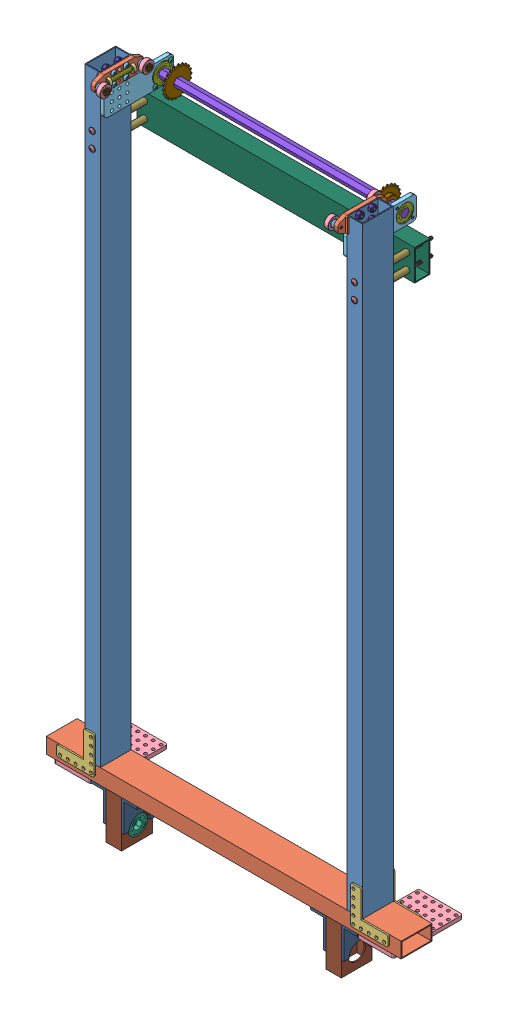
SolidWorks assembly Assem1^short elevator(1), configuration Default. Lengths in mm.
Overall size (584.2 1114.95 169.19).
89 component instances, 24 part files, 69 mates.
Components (placement in the parent):
- 2x1 extrude-1: 2x1 extrude [Default] at (149.0883 176.1618 1108.344) size (25.4 990.6 50.8)
- 2x1 extrude-2: 2x1 extrude [Default] at (580.8883 176.1618 1108.344) size (25.4 990.6 50.8)
- 2x1 23in extrude-1: 2x1 23in extrude [Default] at (669.7883 150.7618 1057.544) x (0 -1 0) z (-1 0 0) size (25.4 50.8 584.2)
- 90Degree L-1: 90Degree L [Default] at (147.322 -398.8739 726.1446) x (0 -1 0) z (-0.754511 0 0.656287) size (61.93 42.53 48.36)
- 90Degree L-2: 90Degree L [Default] at (147.322 -398.8739 779.4446) x (0 -1 0) z (-0.754511 0 0.656287) size (61.93 42.53 48.36)
- 90Degree L-3: 90Degree L [Default] at (31.2526 177.9281 726.1446) x (-1 0 0) z (0 0.754511 0.656287) size (61.93 42.53 48.36)
- 90Degree L-4: 90Degree L [Default] at (31.2526 177.9281 779.4446) x (-1 0 0) z (0 0.754511 0.656287) size (61.93 42.53 48.36)
- elevator motor mount-1: elevator motor mount [Default] at (724.1239 177.9281 1386.4435) x (1 0 0) z (0 0.754511 -0.656287) size (73.03 90.18 79.54)
- elevator motor mount-2: elevator motor mount [Default] at (31.2526 117.5955 1386.4435) x (-1 0 0) z (0 -0.754511 -0.656287) size (73.03 90.18 79.54)
- Copy of axle bracket^Assem1_short elevator(1)-2: Copy of axle bracket^Assem1_short elevator(1) [Default] at (-511.8423 2761.443 1667.3239) x (0.041389 -0.998995 -0.017175) z (0.999131 0.041466 -0.004112) size (40.43 115.12 11.68) (virtual)
  - Top Elevator Bearing Plate - ELEV-DRIVE-002.step-1: Top Elevator Bearing Plate - ELEV-DRIVE-002.step [Default] at (533.5722 545.5094 1067.8534) x (-0.017175 -0.999844 -0.004112) z (0.041389 -0.00482 0.999131) size (114.3 38.1 6.35)
  - 91255A191_Button Head Hex Drive Screw (1).step-1: 91255A191_Button Head Hex Drive Screw (1).step [Default] at (1706.7511 633.6223 1020.9438) x (-0.998995 0.01699 0.041466) z (-0.041389 0.00482 -0.999131) size (7.92 7.92 10.15)
  - 91255A191_Button Head Hex Drive Screw (1).step-2: 91255A191_Button Head Hex Drive Screw (1).step [Default] at (1680.7252 608.4497 1021.9005) x (-0.998995 0.01699 0.041466) z (-0.041389 0.00482 -0.999131) size (7.92 7.92 10.15)
  - TTB-0001_HalfInchHexBearing.step-1: TTB-0001_HalfInchHexBearing.step [Default] at (1693.9487 621.0115 1026.5041) x (-0.952853 -0.301042 0.03802) z (0.300597 -0.953599 -0.017053) size (31.12 7.94 31.12)
- Copy of Copy of Assem12^Assem1_short elevator(1)-2: Copy of Copy of Assem12^Assem1_short elevator(1) [Default] at (1267.2189 -516.8194 1667.3239) x (-0.041389 0.998995 -0.017175) z (-0.999131 -0.041466 -0.004112) size (40.43 115.12 11.68) (virtual)
  - Top Elevator Bearing Plate - ELEV-DRIVE-002.step-1: Top Elevator Bearing Plate - ELEV-DRIVE-002.step [Default] at (533.5722 545.5094 1067.8534) x (-0.017175 -0.999844 -0.004112) z (0.041389 -0.00482 0.999131) size (114.3 38.1 6.35)
  - 91255A191_Button Head Hex Drive Screw (1).step-1: 91255A191_Button Head Hex Drive Screw (1).step [Default] at (1706.7511 633.6223 1020.9438) x (-0.998995 0.01699 0.041466) z (-0.041389 0.00482 -0.999131) size (7.92 7.92 10.15)
  - 91255A191_Button Head Hex Drive Screw (1).step-2: 91255A191_Button Head Hex Drive Screw (1).step [Default] at (1680.7252 608.4497 1021.9005) x (-0.998995 0.01699 0.041466) z (-0.041389 0.00482 -0.999131) size (7.92 7.92 10.15)
  - TTB-0001_HalfInchHexBearing.step-1: TTB-0001_HalfInchHexBearing.step [Default] at (1693.9487 621.0115 1026.5041) x (-0.952853 -0.301042 0.03802) z (0.300597 -0.953599 -0.017053) size (31.12 7.94 31.12)
- 16in .5 hex axle-1: 16in .5 hex axle [Default] at (580.8883 1126.5392 1025.6307) x (0 0.397978 0.917395) z (-1 0 0) size (14.35 13.94 406.4)
- 22t 25chain gear-1: 22t 25chain gear [Default] at (698.6259 1091.6339 2219.5137) x (1 0 0) z (0 -0.367143 -0.930165) size (9.18 48.36 48.44)
- 22t 25chain gear-2: 22t 25chain gear [Default] at (56.7864 420.9907 1995.199) x (-1 0 0) z (0 0.852889 -0.522092) size (9.18 48.36 48.44)
- Copy of Copy (2) of Assem13^Assem1_short elevator(1)-2: Copy of Copy (2) of Assem13^Assem1_short elevator(1) [Default] at (-330.6974 177.9281 779.4446) x (-1 0 0) z (0 0.754511 0.656287) size (76.2 88.34 90.83) (virtual)
  - 1x2x2 L bracket-1: 1x2x2 L bracket [Default] at (-550.7787 227.658 162.0158) x (0 0.754511 0.656287) z (-1 0 0) size (50.8 50.8 25.4)
  - 1x2x3-1: 1x2x3 [Default] at (-514.7107 227.658 162.0158) x (-1 0 0) z (0 -0.754511 -0.656287) size (25.4 76.2 50.8)
  - 1x2x2 L bracket-2: 1x2x2 L bracket [Default] at (-504.0427 265.9872 195.3552) x (0 -0.754511 -0.656287) z (1 0 0) size (50.8 50.8 25.4)
- Copy of Copy of Assem13^Assem1_short elevator(1)-2: Copy of Copy of Assem13^Assem1_short elevator(1) [Default] at (31.2526 177.9281 779.4446) x (-1 0 0) z (0 0.754511 0.656287) size (76.2 88.34 90.83) (virtual)
  - 1x2x2 L bracket-1: 1x2x2 L bracket [Default] at (-550.7787 227.658 162.0158) x (0 0.754511 0.656287) z (-1 0 0) size (50.8 50.8 25.4)
  - 1x2x3-1: 1x2x3 [Default] at (-514.7107 227.658 162.0158) x (-1 0 0) z (0 -0.754511 -0.656287) size (25.4 76.2 50.8)
  - 1x2x2 L bracket-2: 1x2x2 L bracket [Default] at (-504.0427 265.9872 195.3552) x (0 -0.754511 -0.656287) z (1 0 0) size (50.8 50.8 25.4)
- Copy of Copy of Assem15^Assem1_short elevator(1)-2: Copy of Copy of Assem15^Assem1_short elevator(1) [Default] at (1830.9432 2239.2418 1667.3239) x (-0.916906 -0.398734 -0.017175) z (0.398855 -0.917005 -0.004112) size (13.77 134.77 13.77) (virtual)
  - 1.375in Long Aluminum Spacer for Crossbar ELEV-DRIVE-008.step-1: 1.375in Long Aluminum Spacer for Crossbar ELEV-DRIVE-008.step [Default] at (1618.2207 579.6208 597.2661) x (0.999819 -0.017141 -0.008284) z (0.008213 -0.004254 0.999957) size (9.53 34.92 9.53)
  - 5 Inch Long 10-32 Screw 287951.step-1: 5 Inch Long 10-32 Screw 287951.step [Default] at (1618.4098 590.63 597.3114) x (0.999851 -0.017183 0.001798) z (-0.017175 -0.999844 -0.004112) size (11.43 13.19 134.54)
  - 91831A411_18-8 Stainless Steel Nylon-Insert Locknut (2).step-1: 91831A411_18-8 Stainless Steel Nylon-Insert Locknut (2).step [Default] at (1619.2568 639.9364 597.5142) x (0.999849 -0.017186 0.002623) z (-0.002693 -0.004067 0.999988) size (9.53 5.96 11)
- Copy of Copy (2) of Assem15^Assem1_short elevator(1)-2: Copy of Copy (2) of Assem15^Assem1_short elevator(1) [Default] at (1830.9432 2264.6418 1667.3239) x (-0.916906 -0.398734 -0.017175) z (0.398855 -0.917005 -0.004112) size (13.77 134.77 13.77) (virtual)
  - 1.375in Long Aluminum Spacer for Crossbar ELEV-DRIVE-008.step-1: 1.375in Long Aluminum Spacer for Crossbar ELEV-DRIVE-008.step [Default] at (1618.2207 579.6208 597.2661) x (0.999819 -0.017141 -0.008284) z (0.008213 -0.004254 0.999957) size (9.53 34.92 9.53)
  - 5 Inch Long 10-32 Screw 287951.step-1: 5 Inch Long 10-32 Screw 287951.step [Default] at (1618.4098 590.63 597.3114) x (0.999851 -0.017183 0.001798) z (-0.017175 -0.999844 -0.004112) size (11.43 13.19 134.54)
  - 91831A411_18-8 Stainless Steel Nylon-Insert Locknut (2).step-1: 91831A411_18-8 Stainless Steel Nylon-Insert Locknut (2).step [Default] at (1619.2568 639.9364 597.5142) x (0.999849 -0.017186 0.002623) z (-0.002693 -0.004067 0.999988) size (9.53 5.96 11)
- Copy of Copy (3) of Assem15^Assem1_short elevator(1)-2: Copy of Copy (3) of Assem15^Assem1_short elevator(1) [Default] at (1399.1432 2239.2418 1667.3239) x (-0.916906 -0.398734 -0.017175) z (0.398855 -0.917005 -0.004112) size (13.77 134.77 13.77) (virtual)
  - 1.375in Long Aluminum Spacer for Crossbar ELEV-DRIVE-008.step-1: 1.375in Long Aluminum Spacer for Crossbar ELEV-DRIVE-008.step [Default] at (1618.2207 579.6208 597.2661) x (0.999819 -0.017141 -0.008284) z (0.008213 -0.004254 0.999957) size (9.53 34.92 9.53)
  - 5 Inch Long 10-32 Screw 287951.step-1: 5 Inch Long 10-32 Screw 287951.step [Default] at (1618.4098 590.63 597.3114) x (0.999851 -0.017183 0.001798) z (-0.017175 -0.999844 -0.004112) size (11.43 13.19 134.54)
  - 91831A411_18-8 Stainless Steel Nylon-Insert Locknut (2).step-1: 91831A411_18-8 Stainless Steel Nylon-Insert Locknut (2).step [Default] at (1619.2568 639.9364 597.5142) x (0.999849 -0.017186 0.002623) z (-0.002693 -0.004067 0.999988) size (9.53 5.96 11)
- Copy of Copy (4) of Assem15^Assem1_short elevator(1)-2: Copy of Copy (4) of Assem15^Assem1_short elevator(1) [Default] at (1399.1432 2264.6418 1667.3239) x (-0.916906 -0.398734 -0.017175) z (0.398855 -0.917005 -0.004112) size (13.77 134.77 13.77) (virtual)
  - 1.375in Long Aluminum Spacer for Crossbar ELEV-DRIVE-008.step-1: 1.375in Long Aluminum Spacer for Crossbar ELEV-DRIVE-008.step [Default] at (1618.2207 579.6208 597.2661) x (0.999819 -0.017141 -0.008284) z (0.008213 -0.004254 0.999957) size (9.53 34.92 9.53)
  - 5 Inch Long 10-32 Screw 287951.step-1: 5 Inch Long 10-32 Screw 287951.step [Default] at (1618.4098 590.63 597.3114) x (0.999851 -0.017183 0.001798) z (-0.017175 -0.999844 -0.004112) size (11.43 13.19 134.54)
  - 91831A411_18-8 Stainless Steel Nylon-Insert Locknut (2).step-1: 91831A411_18-8 Stainless Steel Nylon-Insert Locknut (2).step [Default] at (1619.2568 639.9364 597.5142) x (0.999849 -0.017186 0.002623) z (-0.002693 -0.004067 0.999988) size (9.53 5.96 11)
- 2x1 18in extrude-1: 2x1 18in extrude [Default] at (149.0883 1090.5618 997.219) x (1 0 0) z (0 -1 0) size (457.2 25.4 50.8)
- Copy of Copy of Assem10^Assem1_short elevator(1)-2: Copy of Copy of Assem10^Assem1_short elevator(1) [Default] at (-527.4189 487.9 -235.3019) x (-1 0 0) z (0 1 0) size (31.06 89.43 29.43) (virtual)
  - Sliding Elevator Bearing Block Kit.step-1: Sliding Elevator Bearing Block Kit.step [Default] at (-2.279 1755.626 148.4607) x (0 -0.999847 -0.017493) z (-1 0 0) size (88.96 27.87 31.06)
    - .25diameter_1.75inSteelDowel_SLIDE-002.step-1: .25diameter_1.75inSteelDowel_SLIDE-002.step [Default] at (428.3334 525.2741 706.1052) x (0.999847 0.017493 0) z (0 0 1) size (44.45 6.35 6.35)
    - 10-32 Locknut 2623.step-1: 10-32 Locknut 2623.step [Default] at (418.0305 533.3501 696.4532) x (1 0 0) z (0 1 0) size (9.53 5.96 11)
    - Bearing Block Shoulder Bolt - SLIDE-004.step-1: Bearing Block Shoulder Bolt - SLIDE-004.step [Default] at (393.4137 524.6631 723.447) x (0.999978 0.006628 0) z (0 0 1) size (9.53 9.53 21.53)
    - Bearing Block Shoulder Bolt Spacer - SLIDE-003.step-1: Bearing Block Shoulder Bolt Spacer - SLIDE-003.step [Default] at (209.8469 202.8854 705.9782) x (0.999977 0.006804 0) z (0 0 1) size (10.72 10.72 5.56)
    - Sliding Bearing Block Plate - SLIDE-001.step-1: Sliding Bearing Block Plate - SLIDE-001.step [Default] at (417.8216 -325.94 699.6282) x (0.999847 0.017493 0) z (0 0 1) size (81.28 25.4 9.54)
    - TTB-0027_.50OD_.25ID_.188WD.step-1: TTB-0027_.50OD_.25ID_.188WD.step [Default] at (448.2757 525.623 706.1052) x (0 0 -1) z (0.999847 0.017493 0) size (12.7 12.7 4.76)
    - TTB-0038_75OD_25ID_28WD.step-1: TTB-0038_75OD_25ID_28WD.step [Default] at (463.253 525.885 715.1127) size (19.05 19.05 7.14)
    - Bearing Block Shoulder Bolt - SLIDE-004.step-2: Bearing Block Shoulder Bolt - SLIDE-004.step [Default] at (463.253 525.885 723.447) size (9.53 9.53 21.53)
    - TTB-0027_.50OD_.25ID_.188WD.step-2: TTB-0027_.50OD_.25ID_.188WD.step [Default] at (408.3911 524.9252 706.1052) x (0 0 -1) z (0.999847 0.017493 0) size (12.7 12.7 4.76)
    - Bearing Block Shoulder Bolt Spacer - SLIDE-003.step-2: Bearing Block Shoulder Bolt Spacer - SLIDE-003.step [Default] at (277.5012 205.3636 705.9782) size (10.72 10.72 5.56)
    - TTB-0038_75OD_25ID_28WD.step-2: TTB-0038_75OD_25ID_28WD.step [Default] at (393.4137 524.6631 715.1127) x (0.999973 0.007362 0) z (0 0 1) size (19.05 19.05 7.14)
    - .625 Long 10-32 Button Head Screw.step-1: .625 Long 10-32 Button Head Screw.step [Default] at (438.3474 533.7055 699.3234) x (0.999998 0.002032 0) z (0 0 1) size (9.17 9.17 18.44)
    - .625 Long 10-32 Button Head Screw.step-2: .625 Long 10-32 Button Head Screw.step [Default] at (438.6362 517.1981 699.3234) x (1 -0.000148 0) z (0 0 1) size (9.17 9.17 18.44)
    - .625 Long 10-32 Button Head Screw.step-3: .625 Long 10-32 Button Head Screw.step [Default] at (418.3193 516.8426 699.3234) x (0.999999 0.001159 0) z (0 0 1) size (9.17 9.17 18.44)
    - .625 Long 10-32 Button Head Screw.step-4: .625 Long 10-32 Button Head Screw.step [Default] at (418.0305 533.3501 699.3234) x (0.999983 0.005862 0) z (0 0 1) size (9.17 9.17 18.44)
    - 10-32 Locknut 2623.step-2: 10-32 Locknut 2623.step [Default] at (438.3474 533.7055 696.4532) x (0.999999 0.001134 0) z (-0.001134 0.999999 0) size (9.53 5.96 11)
    - 10-32 Locknut 2623.step-3: 10-32 Locknut 2623.step [Default] at (438.6362 517.1981 696.4532) x (1 0.000493 0) z (-0.000493 1 0) size (9.53 5.96 11)
    - 10-32 Locknut 2623.step-4: 10-32 Locknut 2623.step [Default] at (418.3193 516.8426 696.4532) x (0.999999 0.001452 0) z (-0.001452 0.999999 0) size (9.53 5.96 11)
- Copy of Copy (2) of Assem10^Assem1_short elevator(1)-2: Copy of Copy (2) of Assem10^Assem1_short elevator(1) [Default] at (1282.7955 1820.2235 -235.1495) x (1 0 0) z (0 -1 0) size (31.06 89.43 29.43) (virtual)
  - Sliding Elevator Bearing Block Kit.step-1: Sliding Elevator Bearing Block Kit.step [Default] at (-2.279 1755.626 148.4607) x (0 -0.999847 -0.017493) z (-1 0 0) size (88.96 27.87 31.06)
    - .25diameter_1.75inSteelDowel_SLIDE-002.step-1: .25diameter_1.75inSteelDowel_SLIDE-002.step [Default] at (428.3334 525.2741 706.1052) x (0.999847 0.017493 0) z (0 0 1) size (44.45 6.35 6.35)
    - 10-32 Locknut 2623.step-1: 10-32 Locknut 2623.step [Default] at (418.0305 533.3501 696.4532) x (1 0 0) z (0 1 0) size (9.53 5.96 11)
    - Bearing Block Shoulder Bolt - SLIDE-004.step-1: Bearing Block Shoulder Bolt - SLIDE-004.step [Default] at (393.4137 524.6631 723.447) x (0.999978 0.006628 0) z (0 0 1) size (9.53 9.53 21.53)
    - Bearing Block Shoulder Bolt Spacer - SLIDE-003.step-1: Bearing Block Shoulder Bolt Spacer - SLIDE-003.step [Default] at (209.8469 202.8854 705.9782) x (0.999977 0.006804 0) z (0 0 1) size (10.72 10.72 5.56)
    - Sliding Bearing Block Plate - SLIDE-001.step-1: Sliding Bearing Block Plate - SLIDE-001.step [Default] at (417.8216 -325.94 699.6282) x (0.999847 0.017493 0) z (0 0 1) size (81.28 25.4 9.54)
    - TTB-0027_.50OD_.25ID_.188WD.step-1: TTB-0027_.50OD_.25ID_.188WD.step [Default] at (448.2757 525.623 706.1052) x (0 0 -1) z (0.999847 0.017493 0) size (12.7 12.7 4.76)
    - TTB-0038_75OD_25ID_28WD.step-1: TTB-0038_75OD_25ID_28WD.step [Default] at (463.253 525.885 715.1127) size (19.05 19.05 7.14)
    - Bearing Block Shoulder Bolt - SLIDE-004.step-2: Bearing Block Shoulder Bolt - SLIDE-004.step [Default] at (463.253 525.885 723.447) size (9.53 9.53 21.53)
    - TTB-0027_.50OD_.25ID_.188WD.step-2: TTB-0027_.50OD_.25ID_.188WD.step [Default] at (408.3911 524.9252 706.1052) x (0 0 -1) z (0.999847 0.017493 0) size (12.7 12.7 4.76)
    - Bearing Block Shoulder Bolt Spacer - SLIDE-003.step-2: Bearing Block Shoulder Bolt Spacer - SLIDE-003.step [Default] at (277.5012 205.3636 705.9782) size (10.72 10.72 5.56)
    - TTB-0038_75OD_25ID_28WD.step-2: TTB-0038_75OD_25ID_28WD.step [Default] at (393.4137 524.6631 715.1127) x (0.999973 0.007362 0) z (0 0 1) size (19.05 19.05 7.14)
    - .625 Long 10-32 Button Head Screw.step-1: .625 Long 10-32 Button Head Screw.step [Default] at (438.3474 533.7055 699.3234) x (0.999998 0.002032 0) z (0 0 1) size (9.17 9.17 18.44)
    - .625 Long 10-32 Button Head Screw.step-2: .625 Long 10-32 Button Head Screw.step [Default] at (438.6362 517.1981 699.3234) x (1 -0.000148 0) z (0 0 1) size (9.17 9.17 18.44)
    - .625 Long 10-32 Button Head Screw.step-3: .625 Long 10-32 Button Head Screw.step [Default] at (418.3193 516.8426 699.3234) x (0.999999 0.001159 0) z (0 0 1) size (9.17 9.17 18.44)
    - .625 Long 10-32 Button Head Screw.step-4: .625 Long 10-32 Button Head Screw.step [Default] at (418.0305 533.3501 699.3234) x (0.999983 0.005862 0) z (0 0 1) size (9.17 9.17 18.44)
    - 10-32 Locknut 2623.step-2: 10-32 Locknut 2623.step [Default] at (438.3474 533.7055 696.4532) x (0.999999 0.001134 0) z (-0.001134 0.999999 0) size (9.53 5.96 11)
    - 10-32 Locknut 2623.step-3: 10-32 Locknut 2623.step [Default] at (438.6362 517.1981 696.4532) x (1 0.000493 0) z (-0.000493 1 0) size (9.53 5.96 11)
    - 10-32 Locknut 2623.step-4: 10-32 Locknut 2623.step [Default] at (418.3193 516.8426 696.4532) x (0.999999 0.001452 0) z (-0.001452 0.999999 0) size (9.53 5.96 11)
- 1.125 with hex bore-1: 1.125 with hex bore [Default] at (1301.5238 -1115.6716 2364.2493) x (-0.00482 0.907617 0.419771) z (-0.999131 -0.021746 0.035545) size (31.12 31.15 9.17)
- 1.125 with hex bore-2: 1.125 with hex bore [Default] at (-546.1472 -834.5964 2581.6464) x (0.00482 -0.634457 -0.772943) z (0.999131 -0.028937 0.029983) size (31.12 31.15 9.17)
Mates (geometry in assembly coordinates):
- Coincident2: coincident aligned: plane of 2x1 extrude-1 through (149.0883 1166.7618 1108.344) normal (0 0 1); plane of 2x1 23in extrude-1 through (85.5883 176.1618 1108.344) normal (0 0 1)
- Perpendicular2: perpendicular: plane of 2x1 extrude-1 through (174.4883 1166.7618 1108.344) normal (1 0 0); plane of 2x1 23in extrude-1 through (85.5883 176.1618 1108.344) normal (0 1 0)
- Coincident4: coincident anti-aligned: plane of 2x1 extrude-1 through (149.0883 176.1618 1108.344) normal (0 -1 0); plane of 2x1 23in extrude-1 through (85.5883 176.1618 1108.344) normal (0 1 0)
- Distance1: distance = 63.5 mm aligned: plane of 2x1 extrude-1 through (149.0883 1166.7618 1108.344) normal (-1 0 0); plane of 2x1 23in extrude-1 through (85.5883 150.7618 1057.544) normal (-1 0 0)
- Coincident17: coincident aligned: plane of 2x1 extrude-1 through (149.0883 1166.7618 1108.344) normal (0 1 0); plane of Copy of Copy of Assem10^Assem1_short elevator(1)-1/Sliding Elevator Bearing Block Kit.step-1/Sliding Bearing Block Plate - SLIDE-001.step-1 through (174.4883 1166.7618 1057.4678) normal (0 1 0)
- Coincident18: coincident anti-aligned: plane of 2x1 extrude-1 through (174.4883 1166.7618 1108.344) normal (1 0 0); plane of Copy of Copy of Assem10^Assem1_short elevator(1)-1/Sliding Elevator Bearing Block Kit.step-1/Sliding Bearing Block Plate - SLIDE-001.step-1 through (174.4883 1154.0618 1082.8678) normal (-1 0 0)
- Coincident19: coincident anti-aligned: plane of 2x1 extrude-1 through (149.0883 1166.7618 1108.344) normal (0 0 1); plane of Copy of Copy of Assem10^Assem1_short elevator(1)-1/Sliding Elevator Bearing Block Kit.step-1/Sliding Bearing Block Plate - SLIDE-001.step-1 through (174.4883 1141.3618 1108.344) normal (0 0 -1)
- Coincident33: coincident aligned: plane of 2x1 extrude-1 through (149.0883 1166.7618 1108.344) normal (-1 0 0); plane of 90Degree L-2 through (149.0883 220.6118 1108.344) normal (-1 0 0)
- Coincident42: coincident anti-aligned: plane of 2x1 extrude-1 through (149.0883 1166.7618 1057.544) normal (0 0 -1); plane of 90Degree L-1 through (135.6009 189.6492 1057.544) normal (0 0 1)
- Coincident44: coincident aligned: plane of 2x1 extrude-1 through (149.0883 1166.7618 1108.344) normal (-1 0 0); plane of 90Degree L-1 through (149.0883 220.6118 1055.044) normal (-1 0 0)
- Coincident92: coincident anti-aligned: plane of 2x1 extrude-1 through (174.4883 1166.7618 1108.344) normal (1 0 0); plane of Copy of Copy of Assem12^Assem1_short elevator(1)-1/Top Elevator Bearing Plate - ELEV-DRIVE-002.step-1 through (174.4883 1122.3118 1051.194) normal (-1 0 0)
- Coincident93: coincident aligned: plane of 2x1 extrude-1 through (149.0883 1166.7618 1108.344) normal (0 0 1); plane of Copy of Copy of Assem12^Assem1_short elevator(1)-1/Top Elevator Bearing Plate - ELEV-DRIVE-002.step-1 through (180.8383 1103.2618 1108.344) normal (0 0 1)
- Coincident108: coincident anti-aligned: plane of 2x1 extrude-1 through (149.0883 1166.7618 1108.344) normal (0 0 1); plane of Copy of Copy (4) of Assem15^Assem1_short elevator(1)-1/5 Inch Long 10-32 Screw 287951.step-1 through (157.6688 1076.0612 1108.344) normal (0 0 -1)
- Distance18: distance = 88.9 mm: cylinder of Copy of Copy (4) of Assem15^Assem1_short elevator(1)-1/1.375in Long Aluminum Spacer for Crossbar ELEV-DRIVE-008.step-1 through (161.7883 1077.8618 1057.544) axis (0 0 -1) radius 4.7625; plane of 2x1 extrude-1 through (149.0883 1166.7618 1108.344) normal (0 1 0)
- Distance19: distance = 12.7 mm: cylinder of Copy of Copy (4) of Assem15^Assem1_short elevator(1)-1/1.375in Long Aluminum Spacer for Crossbar ELEV-DRIVE-008.step-1 through (161.7883 1077.8618 1057.544) axis (0 0 -1) radius 4.7625; plane of 2x1 extrude-1 through (174.4883 1166.7618 1108.344) normal (1 0 0)
- Coincident109: coincident anti-aligned: plane of 2x1 extrude-1 through (149.0883 1166.7618 1108.344) normal (0 0 1); plane of Copy of Copy (3) of Assem15^Assem1_short elevator(1)-1/5 Inch Long 10-32 Screw 287951.step-1 through (157.6688 1050.6612 1108.344) normal (0 0 -1)
- Distance20: distance = 12.7 mm: cylinder of Copy of Copy (3) of Assem15^Assem1_short elevator(1)-1/1.375in Long Aluminum Spacer for Crossbar ELEV-DRIVE-008.step-1 through (161.7883 1052.4618 1057.544) axis (0 0 -1) radius 4.7625; plane of 2x1 extrude-1 through (174.4883 1166.7618 1108.344) normal (1 0 0)
- Coincident6: coincident aligned: plane of 2x1 extrude-2 through (580.8883 1166.7618 1108.344) normal (0 0 1); plane of 2x1 23in extrude-1 through (85.5883 176.1618 1108.344) normal (0 0 1)
- Coincident7: coincident anti-aligned: plane of 2x1 extrude-2 through (580.8883 176.1618 1108.344) normal (0 -1 0); plane of 2x1 23in extrude-1 through (85.5883 176.1618 1108.344) normal (0 1 0)
- Distance2: distance = 63.5 mm aligned: plane of 2x1 23in extrude-1 through (669.7883 150.7618 1057.544) normal (1 0 0); plane of 2x1 extrude-2 through (606.2883 1166.7618 1108.344) normal (1 0 0)
- Coincident20: coincident anti-aligned: plane of 2x1 extrude-2 through (580.8883 1166.7618 1108.344) normal (-1 0 0); plane of Copy of Copy (2) of Assem10^Assem1_short elevator(1)-1/Sliding Elevator Bearing Block Kit.step-1/Sliding Bearing Block Plate - SLIDE-001.step-1 through (580.8883 1154.0618 1083.0202) normal (1 0 0)
- Coincident22: coincident anti-aligned: plane of 2x1 extrude-2 through (580.8883 1166.7618 1057.544) normal (0 0 -1); plane of Copy of Copy (2) of Assem10^Assem1_short elevator(1)-1/Sliding Elevator Bearing Block Kit.step-1/Sliding Bearing Block Plate - SLIDE-001.step-1 through (580.8883 1141.3618 1057.544) normal (0 0 1)
- Coincident23: coincident aligned: plane of 2x1 extrude-2 through (580.8883 1166.7618 1108.344) normal (0 1 0); plane of Copy of Copy (2) of Assem10^Assem1_short elevator(1)-1/Sliding Elevator Bearing Block Kit.step-1/Sliding Bearing Block Plate - SLIDE-001.step-1 through (580.8883 1166.7618 1108.4202) normal (0 1 0)
- Coincident34: coincident anti-aligned: plane of 2x1 extrude-2 through (580.8883 1166.7618 1108.344) normal (0 0 1); plane of 90Degree L-4 through (619.7757 189.6492 1108.344) normal (0 0 -1)
- Coincident36: coincident aligned: plane of 2x1 extrude-2 through (606.2883 1166.7618 1108.344) normal (1 0 0); plane of 90Degree L-4 through (606.2883 176.1618 1108.344) normal (1 0 0)
- Coincident39: coincident anti-aligned: plane of 2x1 extrude-2 through (580.8883 1166.7618 1057.544) normal (0 0 -1); plane of 90Degree L-3 through (619.7757 189.6492 1057.544) normal (0 0 1)
- Coincident40: coincident aligned: plane of 2x1 extrude-2 through (606.2883 1166.7618 1108.344) normal (1 0 0); plane of 90Degree L-3 through (606.2883 176.1618 1055.044) normal (1 0 0)
- Coincident89: coincident anti-aligned: plane of 2x1 extrude-2 through (580.8883 1166.7618 1108.344) normal (-1 0 0); plane of Copy of axle bracket^Assem1_short elevator(1)-1/Top Elevator Bearing Plate - ELEV-DRIVE-002.step-1 through (580.8883 1122.3118 1051.194) normal (1 0 0)
- Coincident91: coincident aligned: plane of 2x1 extrude-2 through (580.8883 1166.7618 1108.344) normal (0 0 1); plane of Copy of axle bracket^Assem1_short elevator(1)-1/Top Elevator Bearing Plate - ELEV-DRIVE-002.step-1 through (574.5383 1141.3618 1108.344) normal (0 0 1)
- Coincident105: coincident anti-aligned: plane of 2x1 extrude-2 through (580.8883 1166.7618 1108.344) normal (0 0 1); plane of Copy of Copy (2) of Assem15^Assem1_short elevator(1)-1/5 Inch Long 10-32 Screw 287951.step-1 through (589.4688 1076.0612 1108.344) normal (0 0 -1)
- Distance14: distance = 88.9 mm: cylinder of Copy of Copy (2) of Assem15^Assem1_short elevator(1)-1/1.375in Long Aluminum Spacer for Crossbar ELEV-DRIVE-008.step-1 through (593.5883 1077.8618 1057.544) axis (0 0 -1) radius 4.7625; line of 2x1 extrude-2 through (580.8883 1166.7618 1108.344) axis (1 0 0)
- Distance15: distance = 12.7 mm: cylinder of Copy of Copy (2) of Assem15^Assem1_short elevator(1)-1/1.375in Long Aluminum Spacer for Crossbar ELEV-DRIVE-008.step-1 through (593.5883 1077.8618 1057.544) axis (0 0 -1) radius 4.7625; plane of 2x1 extrude-2 through (606.2883 1166.7618 1108.344) normal (1 0 0)
- Coincident107: coincident anti-aligned: plane of 2x1 extrude-2 through (580.8883 1166.7618 1108.344) normal (0 0 1); plane of Copy of Copy of Assem15^Assem1_short elevator(1)-1/5 Inch Long 10-32 Screw 287951.step-1 through (589.4688 1050.6612 1108.344) normal (0 0 -1)
- Distance17: distance = 12.7 mm: cylinder of Copy of Copy of Assem15^Assem1_short elevator(1)-1/1.375in Long Aluminum Spacer for Crossbar ELEV-DRIVE-008.step-1 through (593.5883 1052.4618 1057.544) axis (0 0 -1) radius 4.7625; plane of 2x1 extrude-2 through (606.2883 1166.7618 1108.344) normal (1 0 0)
- Coincident111: coincident aligned: plane of 2x1 extrude-2 through (606.2883 1166.7618 1108.344) normal (1 0 0); plane of 2x1 18in extrude-1 through (606.2883 1090.5618 997.219) normal (1 0 0)
- Distance22: distance = 76.2 mm aligned: plane of 2x1 18in extrude-1 through (606.2883 1090.5618 997.219) normal (0 1 0); plane of 2x1 extrude-2 through (580.8883 1166.7618 1108.344) normal (0 1 0)
- Coincident31: coincident aligned: plane of 2x1 23in extrude-1 through (85.5883 176.1618 1108.344) normal (0 1 0); plane of 90Degree L-2 through (149.0883 176.1618 1108.344) normal (0 1 0)
- Coincident32: coincident anti-aligned: plane of 2x1 23in extrude-1 through (85.5883 176.1618 1108.344) normal (0 0 1); plane of 90Degree L-2 through (135.6009 189.6492 1108.344) normal (0 0 -1)
- Coincident37: coincident aligned: plane of 2x1 23in extrude-1 through (85.5883 176.1618 1108.344) normal (0 1 0); plane of 90Degree L-4 through (650.7383 176.1618 1108.344) normal (0 1 0)
- Coincident41: coincident aligned: plane of 2x1 23in extrude-1 through (85.5883 176.1618 1108.344) normal (0 1 0); plane of 90Degree L-3 through (650.7383 176.1618 1055.044) normal (0 1 0)
- Coincident43: coincident aligned: plane of 2x1 23in extrude-1 through (85.5883 176.1618 1108.344) normal (0 1 0); plane of 90Degree L-1 through (149.0883 176.1618 1055.044) normal (0 1 0)
- Coincident75: coincident anti-aligned: plane of 2x1 23in extrude-1 through (85.5883 150.7618 1108.344) normal (0 -1 0); plane of elevator motor mount-1 through (128.4508 150.7618 1051.194) normal (0 1 0)
- Coincident76: coincident aligned: plane of 2x1 23in extrude-1 through (85.5883 176.1618 1108.344) normal (0 0 1); plane of elevator motor mount-1 through (98.2883 144.7618 1108.344) normal (0 0 1)
- Distance12: distance = 12.7 mm aligned: plane of elevator motor mount-1 through (98.2883 144.7618 994.044) normal (-1 0 0); plane of 2x1 23in extrude-1 through (85.5883 150.7618 1057.544) normal (-1 0 0)
- Coincident86: coincident anti-aligned: plane of 2x1 23in extrude-1 through (85.5883 150.7618 1108.344) normal (0 -1 0); plane of elevator motor mount-2 through (626.9258 150.7618 1051.194) normal (0 1 0)
- Distance13: distance = 12.7 mm: plane of 2x1 23in extrude-1 through (669.7883 150.7618 1057.544) normal (1 0 0); line of elevator motor mount-2 through (657.0883 150.7618 997.219) axis (0 0 1)
- Coincident88: coincident aligned: plane of 2x1 23in extrude-1 through (85.5883 176.1618 1108.344) normal (0 0 1); plane of elevator motor mount-2 through (657.0883 150.7618 1108.344) normal (0 0 1)
- Coincident113: coincident anti-aligned: plane of 2x1 23in extrude-1 through (85.5883 150.7618 1108.344) normal (0 -1 0); plane of Copy of Copy of Assem13^Assem1_short elevator(1)-1/1x2x2 L bracket-2 through (545.9633 150.7618 1057.544) normal (0 1 0)
- Coincident115: coincident aligned: plane of 2x1 23in extrude-1 through (85.5883 176.1618 1057.544) normal (0 0 -1); plane of Copy of Copy of Assem13^Assem1_short elevator(1)-1/1x2x3-1 through (545.9633 74.5618 1057.544) normal (0 0 -1)
- Coincident116: coincident anti-aligned: plane of 2x1 23in extrude-1 through (85.5883 150.7618 1108.344) normal (0 -1 0); plane of Copy of Copy (2) of Assem13^Assem1_short elevator(1)-1/1x2x2 L bracket-1 through (209.4133 150.7618 1108.344) normal (0 1 0)
- Coincident118: coincident aligned: plane of 2x1 23in extrude-1 through (85.5883 176.1618 1057.544) normal (0 0 -1); plane of Copy of Copy (2) of Assem13^Assem1_short elevator(1)-1/1x2x3-1 through (184.0133 74.5618 1057.544) normal (0 0 -1)
- Coincident117: coincident anti-aligned: plane of elevator motor mount-1 through (158.6133 144.7618 1108.344) normal (1 0 0); plane of Copy of Copy (2) of Assem13^Assem1_short elevator(1)-1/1x2x2 L bracket-2 through (158.6133 150.7618 1057.544) normal (-1 0 0)
- Coincident114: coincident anti-aligned: plane of elevator motor mount-2 through (596.7633 150.7618 1108.344) normal (-1 0 0); plane of Copy of Copy of Assem13^Assem1_short elevator(1)-1/1x2x2 L bracket-1 through (596.7633 150.7618 1108.344) normal (1 0 0)
- Coincident90: coincident anti-aligned: plane of Copy of Copy (2) of Assem10^Assem1_short elevator(1)-1/Sliding Elevator Bearing Block Kit.step-1/Sliding Bearing Block Plate - SLIDE-001.step-1 through (580.8883 1141.3618 1057.6202) normal (0 -1 0); plane of Copy of axle bracket^Assem1_short elevator(1)-1/Top Elevator Bearing Plate - ELEV-DRIVE-002.step-1 through (574.5383 1141.3618 994.044) normal (0 1 0)
- Coincident95: coincident anti-aligned: plane of Copy of axle bracket^Assem1_short elevator(1)-1/TTB-0001_HalfInchHexBearing.step-1 through (580.8883 1123.7767 1020.2904) normal (0 -0.6627 -0.748885); plane of 16in .5 hex axle-1 through (174.4883 1123.7767 1020.2904) normal (0 0.6627 0.748885)
- Coincident96: coincident anti-aligned: plane of Copy of axle bracket^Assem1_short elevator(1)-1/TTB-0001_HalfInchHexBearing.step-1 through (580.8883 1116.812 1017.9608) normal (0 0.317204 -0.948357); plane of 16in .5 hex axle-1 through (174.4883 1116.823 1017.9645) normal (0 -0.317204 0.948357)
- Coincident98: coincident aligned: plane of Copy of axle bracket^Assem1_short elevator(1)-1/TTB-0001_HalfInchHexBearing.step-1 through (580.8883 1131.4653 1016.1557) normal (1 0 0); plane of 16in .5 hex axle-1 through (580.8883 1126.5392 1025.6307) normal (1 0 0)
- Coincident94: coincident anti-aligned: plane of Copy of Copy of Assem10^Assem1_short elevator(1)-1/Sliding Elevator Bearing Block Kit.step-1/Sliding Bearing Block Plate - SLIDE-001.step-1 through (174.4883 1141.3618 1108.2678) normal (0 -1 0); plane of Copy of Copy of Assem12^Assem1_short elevator(1)-1/Top Elevator Bearing Plate - ELEV-DRIVE-002.step-1 through (180.8383 1141.3618 1108.344) normal (0 1 0)
- Coincident99: coincident anti-aligned: plane of 16in .5 hex axle-1 through (174.4883 1127.8052 1008.2462) normal (0 0.317204 -0.948357); plane of 22t 25chain gear-1 through (557.4423 1120.8376 1005.9157) normal (0 -0.317204 0.948357)
- Coincident100: coincident anti-aligned: plane of 16in .5 hex axle-1 through (174.4883 1129.2678 1015.4312) normal (0 0.979903 -0.199472); plane of 22t 25chain gear-1 through (557.4423 1127.8052 1008.2462) normal (0 -0.979903 0.199472)
- Coincident103: coincident anti-aligned: plane of 16in .5 hex axle-1 through (174.4883 1127.8052 1008.2462) normal (0 0.317204 -0.948357); plane of 22t 25chain gear-2 through (197.97 1127.8191 1008.2509) normal (0 -0.317204 0.948357)
- Coincident104: coincident anti-aligned: plane of 16in .5 hex axle-1 through (174.4883 1120.8515 1005.9204) normal (0 -0.6627 -0.748885); plane of 22t 25chain gear-2 through (197.97 1120.8515 1005.9204) normal (0 0.6627 0.748885)
- Concentric2: concentric aligned: cylinder of Copy of Copy (2) of Assem13^Assem1_short elevator(1)-1/1x2x3-1 through (184.0133 99.9618 1082.944) axis (1 0 0) radius 14.2875; cylinder of 1.125 with hex bore-1 through (203.0633 99.9618 1082.944) axis (1 0 0) radius 14.2748
- Coincident120: coincident anti-aligned: plane of Copy of Copy (2) of Assem13^Assem1_short elevator(1)-1/1x2x3-1 through (209.4133 74.5618 1057.544) normal (1 0 0); plane of 1.125 with hex bore-1 through (209.4133 97.9849 1098.3754) normal (-1 0 0)
- Concentric1: concentric anti-aligned: cylinder of Copy of Copy of Assem13^Assem1_short elevator(1)-1/1x2x3-1 through (545.9633 99.9618 1082.944) axis (1 0 0) radius 14.2875; cylinder of 1.125 with hex bore-2 through (552.3133 99.9618 1082.944) axis (-1 0 0) radius 14.2748
- Coincident119: coincident anti-aligned: plane of Copy of Copy of Assem13^Assem1_short elevator(1)-1/1x2x3-1 through (545.9633 74.5618 1057.544) normal (-1 0 0); plane of 1.125 with hex bore-2 through (545.9633 85.5229 1088.7367) normal (1 0 0)
- Distance16: distance = 25.4 mm: cylinder of Copy of Copy of Assem15^Assem1_short elevator(1)-1/1.375in Long Aluminum Spacer for Crossbar ELEV-DRIVE-008.step-1 through (593.5883 1052.4618 1057.544) axis (0 0 -1) radius 4.7625; cylinder of Copy of Copy (2) of Assem15^Assem1_short elevator(1)-1/1.375in Long Aluminum Spacer for Crossbar ELEV-DRIVE-008.step-1 through (593.5883 1077.8618 1057.544) axis (0 0 -1) radius 4.7625
- Coincident110: coincident anti-aligned: plane of Copy of Copy (2) of Assem15^Assem1_short elevator(1)-1/1.375in Long Aluminum Spacer for Crossbar ELEV-DRIVE-008.step-1 through (593.5883 1077.8618 1022.619) normal (0 0 -1); plane of 2x1 18in extrude-1 through (606.2883 1090.5618 1022.619) normal (0 0 1)
- Distance21: distance = 25.4 mm: cylinder of Copy of Copy (3) of Assem15^Assem1_short elevator(1)-1/1.375in Long Aluminum Spacer for Crossbar ELEV-DRIVE-008.step-1 through (161.7883 1052.4618 1057.544) axis (0 0 -1) radius 4.7625; cylinder of Copy of Copy (4) of Assem15^Assem1_short elevator(1)-1/1.375in Long Aluminum Spacer for Crossbar ELEV-DRIVE-008.step-1 through (161.7883 1077.8618 1057.544) axis (0 0 -1) radius 4.7625
